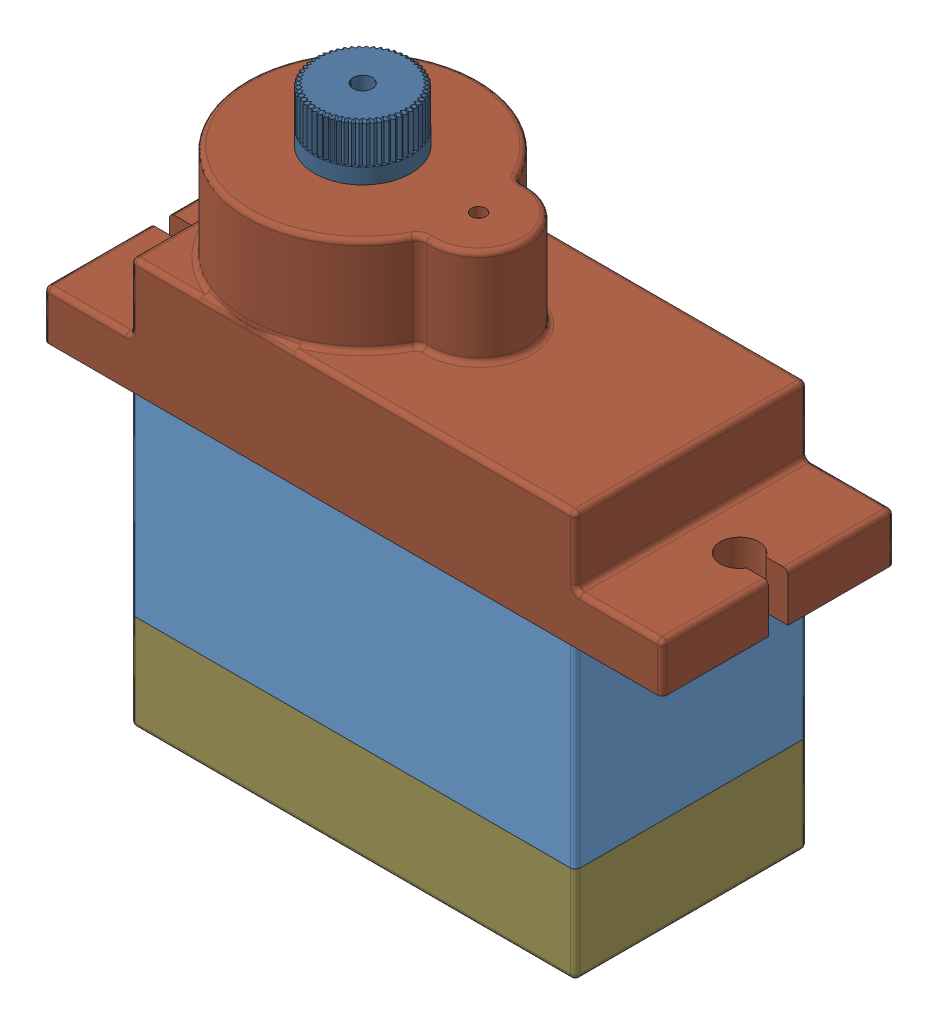
SolidWorks assembly SERVO 2, configuration Default. Lengths in mm.
Overall size (32 28.96 14.19).
25 component instances, 14 part files, 47 mates.
Components (placement in the parent):
- middle cover-1: middle cover [Default] at (8.87 8.8972 15.8774) size (23 11 12)
- shaft-1: shaft [Default] at (3.37 15.3972 15.8774) x (0 1 0) z (-0.985923 0 -0.167197) size (14.5 8.25 8.81)
- part 1-1: part 1 [Default] at (3.37 15.7972 15.8774) x (0 0 1) z (1 0 0) size (9.5 5.14 9.55)
- gear_sub1-1: gear_sub1 [Default] at (9.5 19.3472 15.8774) x (-0.853456 0 0.521165) z (-0.521165 0 -0.853456) size (10.24 10.65 10.25)
  - shaft^gear_sub1-1: shaft^gear_sub1 [Default] at origin size (1 10.65 1) (virtual)
  - spur gear_iso-2: spur gear_iso [ISO - Spur gear 0.25M 39T 20PA 1FW ---S39A75H50L0.8N] at (0 0.1 0) x (0 1 0) z (0 0 1) size (1 10.24 10.25)
  - spur gear_iso-5: spur gear_iso [ISO - Spur gear 0.25M 10T 20PA 1.75FW ---S10A75H50L1.0N] at (0 1.1 0) x (0 1 0) z (0 0 1) size (1.75 2.87 3)
- gear_sub2-1: gear_sub2 [Default] at (3.37 20.7972 15.8774) x (-0.834296 0 0.551317) z (-0.551317 0 -0.834296) size (10.24 2.75 10.25)
  - spur gear_iso-2: spur gear_iso [ISO - Spur gear 0.25M 39T 20PA 1FW ---S39A75H50L0.8N] at (0 0.1 0) x (0 1 0) z (0 0 1) size (1 10.24 10.25)
  - spur gear_iso-5: spur gear_iso [ISO - Spur gear 0.25M 10T 20PA 1.75FW ---S10A75H50L1.0N] at (0 1.1 0) x (0 1 0) z (0 0 1) size (1.75 2.87 3)
- pcb-1: pcb [Default] at (4.7516 11.69 15.8774) x (0.906308 0.422618 0) z (0 0 -1) size (10 2 9)
- wires1^SERVO 2-1: wires1^SERVO 2 [Default] at (8.87 8.8972 21.8774) (virtual)
- DC Motor as part-2: DC Motor as part [Default] at (20.0465 3.7393 19.3612) x (0 0 -1) z (0 1 0) size (8.04 6.55 11.14)
- Rotor scaled-1: Rotor scaled [Default] at (15.62 14.0372 15.8774) x (0.826635 0 -0.562739) z (0 1 0) size (5.2 5.12 15.2)
- spur gear_am-3: spur gear_am [Metric - Spur gear 0.25M 10T 20PA 2FW ---S10N75H50L0.8N] at (15.62 18.9472 15.8774) x (0 1 0) z (0.067436 0 0.997724) size (2 2.87 3)
- gear_sub3-2: gear_sub3 [Default] at (9.5126 21.8914 14.1824) x (-0.43734 0 -0.899296) z (0.899296 0 -0.43734) size (10.24 7 10.25)
  - spur gear_iso-2: spur gear_iso [ISO - Spur gear 0.25M 39T 20PA 1FW ---S39A75H50L0.8N] at (-1.5188 0.3058 -0.7526) x (0 1 0) z (0 0 1) size (1 10.24 10.25)
  - spur gear_iso-6: spur gear_iso [ISO - Spur gear 0.25M 10T 20PA 6FW ---S10A75H50L0.8N] at (-1.5188 1.3058 -0.7526) x (0 1 0) z (0 0 1) size (6 2.87 3)
- gear5-1: gear5 [Default] at (0.4816 -19.0533 15.951) x (0 -1 0) z (0.847043 0 0.531525) size (6.5 10.24 10.25)
- Part5-1: Part5 [Default] at (8.87 24.8972 15.8774) size (32 11 12.1)
- part 3 bottom-1: part 3 bottom [Default] at (8.87 3.8972 15.8774) size (23 5 12)
- Part6-1: Part6 [Default] at (-1.38 3.7472 11.1274) x (0 1 0) z (-0.44899 0 0.893537) size (20.01 2 2)
- Part6-2: Part6 [Default] at (-1.38 3.7472 20.6274) x (0 1 0) z (-0.272553 0 0.962141) size (20.01 2 2)
- Part6-4: Part6 [Default] at (19.12 3.7472 20.6274) x (0 1 0) z (-0.058733 0 0.998274) size (20.01 2 2)
- Part6-6: Part6 [Default] at (19.12 3.7472 11.1274) x (0 1 0) z (0.17693 0 0.984223) size (20.01 2 2)
Mates (geometry in assembly coordinates):
- Concentric1: concentric anti-aligned: cylinder of middle cover-1 through (3.37 8.8962 15.8774) axis (0 1 0) radius 5; cylinder of part 1-1 through (3.37 16.2972 15.8774) axis (0 -1 0) radius 4.75
- Concentric2: concentric aligned: cylinder of shaft-1 through (3.37 15.3972 15.8774) axis (0 -1 0) radius 0.6; cylinder of part 1-1 through (3.37 19.2972 15.8774) axis (0 -1 0) radius 4.5
- Tangent1: tangent: plane of assembly; face of shaft-1; plane of part 1-1 through (4.8064 16.4472 14.6722) normal (0 1 0)
- Concentric3: concentric aligned: cylinder of shaft-1 through (3.37 15.3972 15.8774) axis (0 -1 0) radius 0.5; cylinder of gear_sub2-1/spur gear_iso-5 through (3.37 71.8973 15.8774) axis (0 -1 0) radius 0.5
- Coincident6: coincident anti-aligned: plane of shaft-1 through (3.4536 20.8972 15.3844) normal (0 1 0); plane of gear_sub2-1/spur gear_iso-2 through (3.37 20.8972 15.8774) normal (0 -1 0)
- Concentric4: concentric aligned: cylinder of middle cover-1 through (9.5 19.4472 15.8774) axis (0 -1 0) radius 0.5; cylinder of gear_sub1-1/shaft^gear_sub1-1 through (9.5 18.6972 15.8774) axis (0 -1 0) radius 0.5
- Width1: width anti-aligned: plane of pcb-1 through (9.6001 13.1234 20.3774) normal (0 0 1); plane of pcb-1 through (9.6001 13.1234 11.3774) normal (0 0 -1); plane of middle cover-1 through (20.37 18.8972 20.8774) normal (0 0 -1); plane of middle cover-1 through (20.37 18.8972 10.8774) normal (0 0 1)
- Coincident9: coincident: plane of middle cover-1 through (8.87 8.8972 15.8774) normal (0 -1 0); line of pcb-1 through (0.537 8.8972 20.3774) axis (0 0 -1)
- Angle1: planar angle = 0.436332 rad aligned: plane of pcb-1 through (5.0685 11.0103 15.8774) normal (0.422618 -0.906308 0); plane of middle cover-1 through (8.87 8.8972 15.8774) normal (0 -1 0)
- Tangent2: tangent: cylinder of middle cover-1 through (-1.38 18.8972 20.6274) axis (0 -1 0) radius 1.6; line of pcb-1 through (0.22 9.5769 20.3774) axis (0 0 -1)
- InPlace1: in place: plane of middle cover-1 through (20.37 18.8972 21.8774) normal (0 0 1); plane of ? through (0 0 21.8774) normal (0 0 1); moOrthogonalPlaneRef_w of middle cover-1 through (20.37 18.8972 21.8774) normal (0 0 1); plane of ? through (0 0 21.8774) normal (0 1 0); plane of middle cover-1 through (20.37 18.8972 21.8774) normal (0 0 1); plane of ? through (0 0 21.8774) normal (1 0 0); plane of middle cover-1 through (20.37 18.8972 21.8774) normal (0 0 1); unknown of wires1^SERVO 2-1
- Coincident11: coincident aligned: plane of middle cover-1; plane of wires1^SERVO 2-1
- Coincident12: coincident aligned: moOrthogonalPlaneRef_w of middle cover-1 through (8.87 8.8972 21.8774) normal (0 1 0); plane of wires1^SERVO 2-1 through (8.87 8.8972 21.8774) normal (0 1 0)
- Coincident13: coincident anti-aligned: moOrthogonalPlaneRef_w of middle cover-1 through (8.87 8.8972 21.8774) normal (-1 0 0); plane of wires1^SERVO 2-1 through (8.87 8.8972 21.8774) normal (1 0 0)
- Concentric5: concentric aligned: cylinder of middle cover-1 through (15.62 8.8962 15.8774) axis (0 1 0) radius 1.55; cylinder of DC Motor as part-2 through (15.62 17.7472 15.8774) axis (0 1 0) radius 0.4
- Parallel5: parallel anti-aligned: plane of middle cover-1 through (12.22 12.8972 19.2524) normal (1 0 0); plane of DC Motor as part-2 through (12.62 17.8972 18.5231) normal (-1 0 0)
- Coincident11: coincident anti-aligned: plane of middle cover-1 through (8.87 17.8972 15.8774) normal (0 -1 0); plane of DC Motor as part-2 through (15.62 17.8972 15.8774) normal (0 1 0)
- Coincident12: coincident anti-aligned: circle of DC Motor as part-2; cylinder of Rotor scaled-1 through (15.62 21.6372 15.8774) axis (0 -1 0) radius 0.4
- Coincident13: coincident aligned: plane of DC Motor as part-2 through (14.486 9.2572 14.5254) normal (0 -1 0); plane of Rotor scaled-1 through (15.62 9.2572 15.8774) normal (0 -1 0)
- Coincident15: coincident anti-aligned: plane of middle cover-1 through (8.87 15.2972 15.8774) normal (0 1 0); plane of part 1-1 through (3.37 15.2972 15.8774) normal (0 -1 0)
- Parallel7: parallel aligned: plane of middle cover-1 through (4.62 14.7972 10.8774) normal (1 0 0); plane of part 1-1 through (4.37 15.2972 15.8774) normal (1 0 0)
- Concentric7: concentric aligned: cylinder of Rotor scaled-1 through (15.62 21.6372 15.8774) axis (0 -1 0) radius 0.4; cylinder of spur gear_am-3 through (15.62 68.9473 15.8774) axis (0 -1 0) radius 0.4
- Width2: width aligned: plane of gear_sub1-1/spur gear_iso-2 through (9.5 20.4472 15.8774) normal (0 1 0); plane of gear_sub1-1/spur gear_iso-2 through (9.5 19.4472 15.8774) normal (0 -1 0); plane of spur gear_am-3 through (15.62 20.9472 15.8774) normal (0 1 0); plane of spur gear_am-3 through (15.62 18.9472 15.8774) normal (0 -1 0)
- Lock1: lock: unknown of Rotor scaled-1; unknown of spur gear_am-3
- Concentric8: concentric anti-aligned: cylinder of gear_sub1-1/shaft^gear_sub1-1 through (9.5 18.6972 15.8774) axis (0 1 0) radius 0.5; cylinder of gear_sub3-2/spur gear_iso-6 through (9.5 73.1973 15.8774) axis (0 -1 0) radius 0.4
- Coincident16: coincident anti-aligned: plane of gear_sub1-1/spur gear_iso-5 through (9.5 22.1972 15.8774) normal (0 1 0); plane of gear_sub3-2/spur gear_iso-2 through (9.5 22.1972 15.8774) normal (0 -1 0)
- Concentric9: concentric anti-aligned: cylinder of shaft-1 through (3.37 15.3972 15.8774) axis (0 -1 0) radius 0.6; cylinder of gear5-1 through (3.37 -20.8028 15.8774) axis (0 1 0) radius 0.5
- GearMate5: gear = 39 : 10 mm: cylinder of spur gear_am-3 through (15.62 20.9472 15.8774) axis (0 -1 0) radius 0.9365; cylinder of gear_sub1-1/spur gear_iso-2 through (9.5 20.4472 15.8774) axis (0 -1 0) radius 4.5615
- GearMate6: gear = 39 : 10 mm: cylinder of gear_sub1-1/spur gear_iso-5 through (9.5 22.1972 15.8774) axis (0 -1 0) radius 0.9365; cylinder of gear_sub2-1/spur gear_iso-2 through (3.37 21.8972 15.8774) axis (0 -1 0) radius 4.5615
- GearMate7: gear = 39 : 10 mm: cylinder of gear_sub2-1/spur gear_iso-5 through (3.37 23.6472 15.8774) axis (0 -1 0) radius 0.9365; cylinder of gear_sub3-2/spur gear_iso-2 through (9.5 23.1972 15.8774) axis (0 -1 0) radius 4.5615
- GearMate8: gear = 39 : 10 mm: cylinder of gear_sub3-2/spur gear_iso-6 through (9.5 29.1972 15.8774) axis (0 -1 0) radius 0.9365; cylinder of gear5-1 through (3.37 26.1972 15.8774) axis (0 1 0) radius 4.5615
- Coincident17: coincident aligned: plane of gear_sub3-2/spur gear_iso-6 through (9.5 29.1972 15.8774) normal (0 1 0); plane of gear5-1 through (3.37 29.1972 15.8774) normal (0 1 0)
- Lock3: lock: unknown of shaft-1; unknown of gear5-1
- Concentric11: concentric anti-aligned: cylinder of middle cover-1 through (-1.38 19.8972 20.6274) axis (0 -1 0) radius 1; cylinder of Part5-1 through (-1.38 18.8972 20.6274) axis (0 1 0) radius 1
- Concentric12: concentric anti-aligned: cylinder of middle cover-1 through (19.12 19.8972 11.1274) axis (0 -1 0) radius 1; cylinder of Part5-1 through (19.12 18.8972 11.1274) axis (0 1 0) radius 1
- Coincident18: coincident anti-aligned: plane of middle cover-1 through (8.87 18.8972 15.8774) normal (0 1 0); plane of Part5-1 through (8.87 18.8972 15.8774) normal (0 -1 0)
- Coincident19: coincident anti-aligned: plane of middle cover-1 through (8.87 8.8972 15.8774) normal (0 -1 0); plane of part 3 bottom-1 through (8.87 8.8972 15.8774) normal (0 1 0)
- Concentric13: concentric aligned: cylinder of middle cover-1 through (-1.38 18.8972 20.6274) axis (0 -1 0) radius 0.6; cylinder of part 3 bottom-1 through (-1.38 8.8972 20.6274) axis (0 -1 0) radius 1
- Concentric14: concentric aligned: cylinder of middle cover-1 through (19.12 18.8972 20.6274) axis (0 -1 0) radius 0.6; cylinder of part 3 bottom-1 through (19.12 8.8972 20.6274) axis (0 -1 0) radius 1
- Concentric16: concentric aligned: cylinder of part 3 bottom-1 through (-1.38 7.2472 11.1274) axis (0 -1 0) radius 0.6; cylinder of Part6-1 through (-1.38 3.7472 11.1274) axis (0 -1 0) radius 0.5
- Coincident22: coincident anti-aligned: plane of part 3 bottom-1 through (-1.38 4.7472 11.1274) normal (0 -1 0); plane of Part6-1 through (-1.8267 4.7472 10.9029) normal (0 1 0)
- Concentric17: concentric aligned: cylinder of part 3 bottom-1 through (-1.38 7.2472 20.6274) axis (0 -1 0) radius 0.6; cylinder of Part6-2 through (-1.38 3.7472 20.6274) axis (0 -1 0) radius 0.5
- Coincident23: coincident anti-aligned: plane of part 3 bottom-1 through (-1.38 4.7472 20.6274) normal (0 -1 0); plane of Part6-2 through (-1.861 4.7472 20.4911) normal (0 1 0)
- Concentric18: concentric aligned: cylinder of part 3 bottom-1 through (19.12 7.2472 20.6274) axis (0 -1 0) radius 0.6; cylinder of Part6-4 through (19.12 3.7472 20.6274) axis (0 -1 0) radius 0.5
- Coincident24: coincident anti-aligned: plane of part 3 bottom-1 through (19.12 4.7472 20.6274) normal (0 -1 0); plane of Part6-4 through (18.6209 4.7472 20.598) normal (0 1 0)
- Concentric19: concentric aligned: cylinder of part 3 bottom-1 through (19.12 7.2472 11.1274) axis (0 -1 0) radius 0.6; cylinder of Part6-6 through (19.12 3.7472 11.1274) axis (0 -1 0) radius 0.5
- Coincident25: coincident anti-aligned: plane of part 3 bottom-1 through (19.12 4.7472 11.1274) normal (0 -1 0); plane of Part6-6 through (18.6279 4.7472 11.2158) normal (0 1 0)
